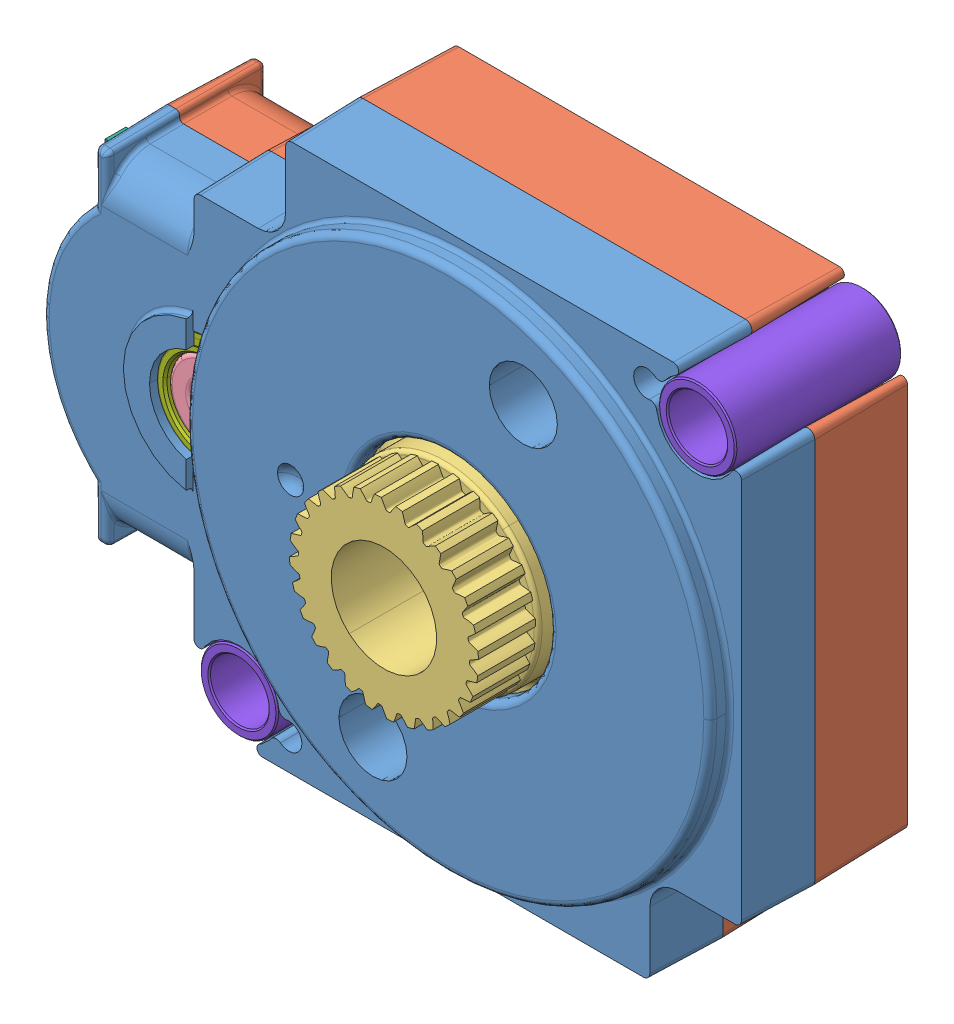
SolidWorks assembly VersaPlanetary Integrated Encoder (217-5046).step, configuration Default. Lengths in mm.
Overall size (56.84 43.13 21.21).
11 component instances, 10 part files, 0 mates.
Components (placement in the parent):
- 217-4783-001 Rev3.step-1: 217-4783-001 Rev3.step [Default] at (0 0 2.75) size (53.55 42 10.7)
- 217-4783-002 Rev7_Sealed Config.step-1: 217-4783-002 Rev7_Sealed Config.step [Default] at (0 0 -7.2) x (0 1 0) z (0 0 1) size (42 51.57 9.32)
- 217-4783-005 Rev7_40t_spur_REF_14deg.step-1: 217-4783-005 Rev7_40t_spur_REF_14deg.step [Default] at (0 0 5.95) x (0.660339 0.750968 0) z (0 0 1) size (21.02 21.02 17.1)
- 217-4783-004 Rev2_40t_spur_REF_14deg.step-1: 217-4783-004 Rev2_40t_spur_REF_14deg.step [Default] at (-20.05 0 5.2) x (-0.718289 0.695745 0) z (0 0 1) size (20.97 20.97 4.88)
- 217-4783-008 Rev2.step-1: 217-4783-008 Rev2.step [Default] at (-20.05 0 2.2) x (0.307149 -0.951661 0) z (0.951661 0.307149 0) size (5 4 5)
- PCBA Rev3.step-1: PCBA Rev3.step [Default] at (-20.05 0 -2.1252) x (0 1 0) z (-1 0 0) size (15.94 8.71 23.22)
- 217-2788-001 Rev3_57155K375.step-1: 217-2788-001 Rev3_57155K375.step [Default] at (-20.05 0 3.8125) x (-0.99574 0.092202 0) z (0 0 1) size (9.53 9.53 3.17)
- 217-4783-006 Rev3.step-1: 217-4783-006 Rev3.step [Default] at (17.5 17.5 -0.85) x (-0.867641 0.497191 0) z (0 0 1) size (5.9 5.9 12.7)
- 217-4783-006 Rev3.step-2: 217-4783-006 Rev3.step [Default] at (-17.5 -17.5 -0.85) x (0.825154 -0.564908 0) z (0 0 1) size (5.9 5.9 12.7)
- 217-4783-007 Rev1.step-1: 217-4783-007 Rev1.step [Default] at (-16.45 0 -5.2) x (0 1 0) z (0 0 1) size (6 10.71 3.51)
- 217-4783-003 Rev4.step-1: 217-4783-003 Rev4.step [Default] at (-20.05 0 -1.02) x (0 1 0) z (0 0 1) size (23.4 21.71 4.29)
